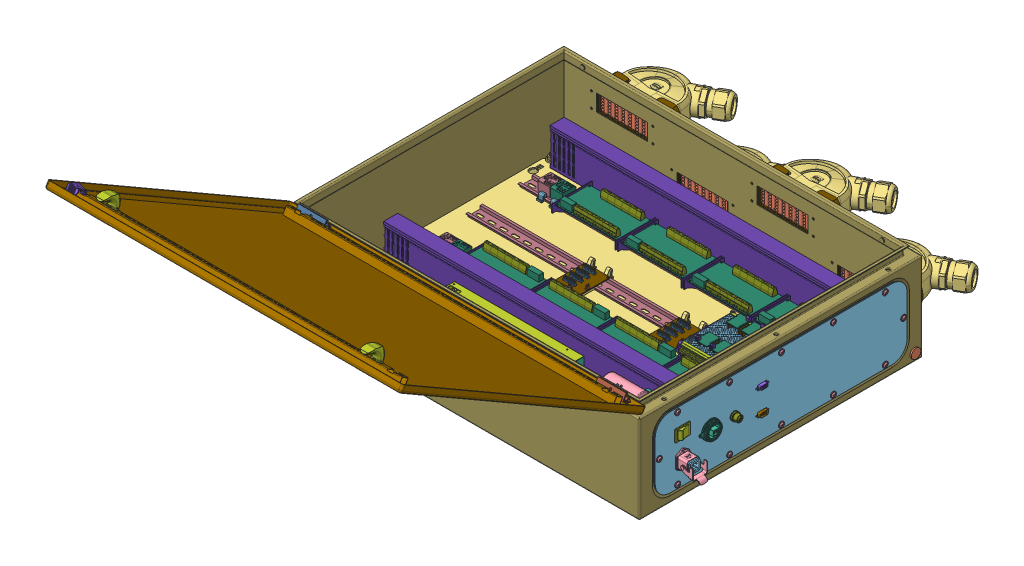
SolidWorks assembly _main_cabinet, configuration Default. Lengths in mm.
Overall size (807.06 524.8 1268.8).
399 component instances, 81 part files, 82 mates.
Components (placement in the parent):
- 1076_000_1_customized-1: 1076_000_1_customized [Default] x (0 0 -1) z (0 1 0) size (1110.24 763.7 524.8)
  - 1076_000_1__3-1: 1076_000_1__3 [Default] at (-280 360 -1.55) x (1 0 0) z (0 0 -1) size (15.5 15.5 6.5)
  - 1076_000_1__3-2: 1076_000_1__3 [Default] at (280 360 -1.55) x (1 0 0) z (0 0 -1) size (15.5 15.5 6.5)
  - 1076_000_1__3-3: 1076_000_1__3 [Default] at (-280 -360 -1.55) x (1 0 0) z (0 0 -1) size (15.5 15.5 6.5)
  - 1076_000_1__3-4: 1076_000_1__3 [Default] at (280 -360 -1.55) x (1 0 0) z (0 0 -1) size (15.5 15.5 6.5)
  - 1076_000_1__8-1: 1076_000_1__8 [Default] at (283.5 -380 16.5) size (20 6.85 20)
  - 1076_000_1__10-1: 1076_000_1__10 [Default] at (0 -355 20) size (550 735 2.5)
  - 1076_000_1__12-1: 1076_000_1__12 [Default] at (220 -379.25 160) x (1 0 0) z (0 0 -1) size (11.5 13.2 11.5)
  - 1076_000_1__12-2: 1076_000_1__12 [Default] at (110 -379.25 160) x (1 0 0) z (0 0 -1) size (11.5 13.2 11.5)
  - 1076_000_1__12-3: 1076_000_1__12 [Default] at (0 -379.25 160) x (1 0 0) z (0 0 -1) size (11.5 13.2 11.5)
  - 1076_000_1__12-4: 1076_000_1__12 [Default] at (-110 -379.25 160) x (1 0 0) z (0 0 -1) size (11.5 13.2 11.5)
  - 1076_000_1__12-5: 1076_000_1__12 [Default] at (-220 -379.25 160) x (1 0 0) z (0 0 -1) size (11.5 13.2 11.5)
  - 1076_000_1__12-6: 1076_000_1__12 [Default] at (220 -379.25 27) x (1 0 0) z (0 0 -1) size (11.5 13.2 11.5)
  - 1076_000_1__12-7: 1076_000_1__12 [Default] at (110 -379.25 27) x (1 0 0) z (0 0 -1) size (11.5 13.2 11.5)
  - 1076_000_1__12-8: 1076_000_1__12 [Default] at (0 -379.25 27) x (1 0 0) z (0 0 -1) size (11.5 13.2 11.5)
  - 1076_000_1__12-9: 1076_000_1__12 [Default] at (-110 -379.25 27) x (1 0 0) z (0 0 -1) size (11.5 13.2 11.5)
  - 1076_000_1__12-10: 1076_000_1__12 [Default] at (-220 -379.25 27) x (1 0 0) z (0 0 -1) size (11.5 13.2 11.5)
  - 1076_000_1__12-11: 1076_000_1__12 [Default] at (259 -379.25 93.5) x (1 0 0) z (0 0 -1) size (11.5 13.2 11.5)
  - 1076_000_1__12-12: 1076_000_1__12 [Default] at (-259 -379.25 93.5) x (1 0 0) z (0 0 -1) size (11.5 13.2 11.5)
  - 1076_000_1__25_customized-1: 1076_000_1__25_customized [Default] at (0 -380.5 93.5) size (534 1.5 149)
  - 1076_000_1__27-1: 1076_000_1__27 [Default] at (-278 -317.5 194.75) x (0 0 -1) z (0 1 0) size (10 7.19 10)
  - 1076_000_1__27-2: 1076_000_1__27 [Default] at (-278 317.5 194.75) x (0 0 -1) z (0 1 0) size (10 7.19 10)
  - Door^1076_000_1_customized-1: Door^1076_000_1_customized [Default] at (-443.434 0 518.2603) x (0.866025 0 -0.5) z (-0.5 0 -0.866025) size (595 755 52.01) (virtual)
    - 1076_000_1__30-1: 1076_000_1__30 [Default] at (-249.348 -280 210.722) x (1 0 0) z (0 -1 0) size (55.65 52.01 55.1)
    - 1076_000_1__30-2: 1076_000_1__30 [Default] at (-249.348 280 210.722) x (1 0 0) z (0 -1 0) size (55.65 52.01 55.1)
    - 1076_000_1__33-1: 1076_000_1__33 [Default] at (-262.098 -333 201.672) x (-1 0 0) z (0 0 -1) size (20.91 29.5 13.98)
    - 1076_000_1__35-1: 1076_000_1__35 [Default] at (-0.1395 1.3759 210.2049) size (595 755 17.5)
    - 1076_000_1__37-1: 1076_000_1__37 [Default] at (279.5 -317.5 194.75) x (0 0 1) z (1 0 0) size (16.07 66 15.75)
    - 1076_000_1__39-1: 1076_000_1__39 [Default] at (279.5 317.5 194.75) x (0 0 1) z (1 0 0) size (16.07 66 15.75)
  - 1076_000_1__41_customized-1: 1076_000_1__41_customized [Default] at (0 -380 105) size (600 760 205.1)
- DIN_rail_35x7.5_long-1: DIN_rail_35x7.5_long [Default] at (-340 20 -70) x (0 0 -1) z (1 0 0) size (35 7.5 680)
- DIN_rail_35x7.5_long-2: DIN_rail_35x7.5_long [Default] at (-340 20 -180) x (0 0 -1) z (1 0 0) size (35 7.5 680)
- DIN_rail_35x7.5_long-3: DIN_rail_35x7.5_long [Default] at (-340 20 40) x (0 0 -1) z (1 0 0) size (35 7.5 680)
- DIN_rail_35x7.5_psus-1: DIN_rail_35x7.5_psus [Default] at (247.5 20 125) size (35 7.5 150)
- Sanwo_16ch_mosfet_board-1: Sanwo_16ch_mosfet_board [Default] at (-242.3811 45.9 -143.9) size (136.5 36.9 85)
  - Sanwo_16ch_mosfet_board-1: Sanwo_16ch_mosfet_board [Default] at origin size (133.5 14.6 72.2)
  - screw_terminal_3x_large-1: screw_terminal_3x_large [Default] at (73.5 1.6 -64.7) size (15 18 10)
  - screw_terminal_3x_large-2: screw_terminal_3x_large [Default] at (103.5 1.6 -64.7) size (15 18 10)
  - screw_terminal_3x_large-3: screw_terminal_3x_large [Default] at (88.5 1.6 -64.7) size (15 18 10)
  - screw_terminal_3x_large-4: screw_terminal_3x_large [Default] at (58.5 1.6 -64.7) size (15 18 10)
  - screw_terminal_3x_large-5: screw_terminal_3x_large [Default] at (113.5 1.6 -64.7) size (15 18 10)
  - screw_terminal_3x_large-6: screw_terminal_3x_large [Default] at (43.5 1.6 -64.7) size (15 18 10)
  - screw_terminal_3x_large-7: screw_terminal_3x_large [Default] at (43.5 1.6 -7.5) x (-1 0 0) z (0 0 -1) size (15 18 10)
  - screw_terminal_3x_large-8: screw_terminal_3x_large [Default] at (103.5 1.6 -7.5) x (-1 0 0) z (0 0 -1) size (15 18 10)
  - screw_terminal_3x_large-9: screw_terminal_3x_large [Default] at (118.5 1.6 -7.5) x (-1 0 0) z (0 0 -1) size (15 18 10)
  - screw_terminal_3x_large-10: screw_terminal_3x_large [Default] at (73.5 1.6 -7.5) x (-1 0 0) z (0 0 -1) size (15 18 10)
  - screw_terminal_3x_large-11: screw_terminal_3x_large [Default] at (58.5 1.6 -7.5) x (-1 0 0) z (0 0 -1) size (15 18 10)
  - screw_terminal_3x_large-12: screw_terminal_3x_large [Default] at (88.5 1.6 -7.5) x (-1 0 0) z (0 0 -1) size (15 18 10)
  - Sanwo_16ch_mosfet_board_DIN_rail_support-1: Sanwo_16ch_mosfet_board_DIN_rail_support [Default] at (0 -18.4 -36.1) x (0 0 1) z (-1 0 0) size (85 26.2 1.5)
  - Sanwo_16ch_mosfet_board_DIN_rail_support-2: Sanwo_16ch_mosfet_board_DIN_rail_support [Default] at (135 -18.4 -36.1) x (0 0 1) z (-1 0 0) size (85 26.2 1.5)
- Sanwo_16ch_mosfet_board-2: Sanwo_16ch_mosfet_board [Default] at (-108.8811 45.9 3.9) x (-1 0 0) z (0 0 -1) size (136.5 36.9 85)
  - Sanwo_16ch_mosfet_board-1: Sanwo_16ch_mosfet_board [Default] at origin size (133.5 14.6 72.2)
  - screw_terminal_3x_large-1: screw_terminal_3x_large [Default] at (73.5 1.6 -64.7) size (15 18 10)
  - screw_terminal_3x_large-2: screw_terminal_3x_large [Default] at (103.5 1.6 -64.7) size (15 18 10)
  - screw_terminal_3x_large-3: screw_terminal_3x_large [Default] at (88.5 1.6 -64.7) size (15 18 10)
  - screw_terminal_3x_large-4: screw_terminal_3x_large [Default] at (58.5 1.6 -64.7) size (15 18 10)
  - screw_terminal_3x_large-5: screw_terminal_3x_large [Default] at (113.5 1.6 -64.7) size (15 18 10)
  - screw_terminal_3x_large-6: screw_terminal_3x_large [Default] at (43.5 1.6 -64.7) size (15 18 10)
  - screw_terminal_3x_large-7: screw_terminal_3x_large [Default] at (43.5 1.6 -7.5) x (-1 0 0) z (0 0 -1) size (15 18 10)
  - screw_terminal_3x_large-8: screw_terminal_3x_large [Default] at (103.5 1.6 -7.5) x (-1 0 0) z (0 0 -1) size (15 18 10)
  - screw_terminal_3x_large-9: screw_terminal_3x_large [Default] at (118.5 1.6 -7.5) x (-1 0 0) z (0 0 -1) size (15 18 10)
  - screw_terminal_3x_large-10: screw_terminal_3x_large [Default] at (73.5 1.6 -7.5) x (-1 0 0) z (0 0 -1) size (15 18 10)
  - screw_terminal_3x_large-11: screw_terminal_3x_large [Default] at (58.5 1.6 -7.5) x (-1 0 0) z (0 0 -1) size (15 18 10)
  - screw_terminal_3x_large-12: screw_terminal_3x_large [Default] at (88.5 1.6 -7.5) x (-1 0 0) z (0 0 -1) size (15 18 10)
  - Sanwo_16ch_mosfet_board_DIN_rail_support-1: Sanwo_16ch_mosfet_board_DIN_rail_support [Default] at (0 -18.4 -36.1) x (0 0 1) z (-1 0 0) size (85 26.2 1.5)
  - Sanwo_16ch_mosfet_board_DIN_rail_support-2: Sanwo_16ch_mosfet_board_DIN_rail_support [Default] at (135 -18.4 -36.1) x (0 0 1) z (-1 0 0) size (85 26.2 1.5)
- Sanwo_16ch_mosfet_board-3: Sanwo_16ch_mosfet_board [Default] at (31.1189 45.9 3.9) x (-1 0 0) z (0 0 -1) size (136.5 36.9 85)
  - Sanwo_16ch_mosfet_board-1: Sanwo_16ch_mosfet_board [Default] at origin size (133.5 14.6 72.2)
  - screw_terminal_3x_large-1: screw_terminal_3x_large [Default] at (73.5 1.6 -64.7) size (15 18 10)
  - screw_terminal_3x_large-2: screw_terminal_3x_large [Default] at (103.5 1.6 -64.7) size (15 18 10)
  - screw_terminal_3x_large-3: screw_terminal_3x_large [Default] at (88.5 1.6 -64.7) size (15 18 10)
  - screw_terminal_3x_large-4: screw_terminal_3x_large [Default] at (58.5 1.6 -64.7) size (15 18 10)
  - screw_terminal_3x_large-5: screw_terminal_3x_large [Default] at (113.5 1.6 -64.7) size (15 18 10)
  - screw_terminal_3x_large-6: screw_terminal_3x_large [Default] at (43.5 1.6 -64.7) size (15 18 10)
  - screw_terminal_3x_large-7: screw_terminal_3x_large [Default] at (43.5 1.6 -7.5) x (-1 0 0) z (0 0 -1) size (15 18 10)
  - screw_terminal_3x_large-8: screw_terminal_3x_large [Default] at (103.5 1.6 -7.5) x (-1 0 0) z (0 0 -1) size (15 18 10)
  - screw_terminal_3x_large-9: screw_terminal_3x_large [Default] at (118.5 1.6 -7.5) x (-1 0 0) z (0 0 -1) size (15 18 10)
  - screw_terminal_3x_large-10: screw_terminal_3x_large [Default] at (73.5 1.6 -7.5) x (-1 0 0) z (0 0 -1) size (15 18 10)
  - screw_terminal_3x_large-11: screw_terminal_3x_large [Default] at (58.5 1.6 -7.5) x (-1 0 0) z (0 0 -1) size (15 18 10)
  - screw_terminal_3x_large-12: screw_terminal_3x_large [Default] at (88.5 1.6 -7.5) x (-1 0 0) z (0 0 -1) size (15 18 10)
  - Sanwo_16ch_mosfet_board_DIN_rail_support-1: Sanwo_16ch_mosfet_board_DIN_rail_support [Default] at (0 -18.4 -36.1) x (0 0 1) z (-1 0 0) size (85 26.2 1.5)
  - Sanwo_16ch_mosfet_board_DIN_rail_support-2: Sanwo_16ch_mosfet_board_DIN_rail_support [Default] at (135 -18.4 -36.1) x (0 0 1) z (-1 0 0) size (85 26.2 1.5)
- Sanwo_16ch_mosfet_board-4: Sanwo_16ch_mosfet_board [Default] at (171.1189 45.9 3.9) x (-1 0 0) z (0 0 -1) size (136.5 36.9 85)
  - Sanwo_16ch_mosfet_board-1: Sanwo_16ch_mosfet_board [Default] at origin size (133.5 14.6 72.2)
  - screw_terminal_3x_large-1: screw_terminal_3x_large [Default] at (73.5 1.6 -64.7) size (15 18 10)
  - screw_terminal_3x_large-2: screw_terminal_3x_large [Default] at (103.5 1.6 -64.7) size (15 18 10)
  - screw_terminal_3x_large-3: screw_terminal_3x_large [Default] at (88.5 1.6 -64.7) size (15 18 10)
  - screw_terminal_3x_large-4: screw_terminal_3x_large [Default] at (58.5 1.6 -64.7) size (15 18 10)
  - screw_terminal_3x_large-5: screw_terminal_3x_large [Default] at (113.5 1.6 -64.7) size (15 18 10)
  - screw_terminal_3x_large-6: screw_terminal_3x_large [Default] at (43.5 1.6 -64.7) size (15 18 10)
  - screw_terminal_3x_large-7: screw_terminal_3x_large [Default] at (43.5 1.6 -7.5) x (-1 0 0) z (0 0 -1) size (15 18 10)
  - screw_terminal_3x_large-8: screw_terminal_3x_large [Default] at (103.5 1.6 -7.5) x (-1 0 0) z (0 0 -1) size (15 18 10)
  - screw_terminal_3x_large-9: screw_terminal_3x_large [Default] at (118.5 1.6 -7.5) x (-1 0 0) z (0 0 -1) size (15 18 10)
  - screw_terminal_3x_large-10: screw_terminal_3x_large [Default] at (73.5 1.6 -7.5) x (-1 0 0) z (0 0 -1) size (15 18 10)
  - screw_terminal_3x_large-11: screw_terminal_3x_large [Default] at (58.5 1.6 -7.5) x (-1 0 0) z (0 0 -1) size (15 18 10)
  - screw_terminal_3x_large-12: screw_terminal_3x_large [Default] at (88.5 1.6 -7.5) x (-1 0 0) z (0 0 -1) size (15 18 10)
  - Sanwo_16ch_mosfet_board_DIN_rail_support-1: Sanwo_16ch_mosfet_board_DIN_rail_support [Default] at (0 -18.4 -36.1) x (0 0 1) z (-1 0 0) size (85 26.2 1.5)
  - Sanwo_16ch_mosfet_board_DIN_rail_support-2: Sanwo_16ch_mosfet_board_DIN_rail_support [Default] at (135 -18.4 -36.1) x (0 0 1) z (-1 0 0) size (85 26.2 1.5)
- Sanwo_16ch_mosfet_board-5: Sanwo_16ch_mosfet_board [Default] at (311.1189 45.9 3.9) x (-1 0 0) z (0 0 -1) size (136.5 36.9 85)
  - Sanwo_16ch_mosfet_board-1: Sanwo_16ch_mosfet_board [Default] at origin size (133.5 14.6 72.2)
  - screw_terminal_3x_large-1: screw_terminal_3x_large [Default] at (73.5 1.6 -64.7) size (15 18 10)
  - screw_terminal_3x_large-2: screw_terminal_3x_large [Default] at (103.5 1.6 -64.7) size (15 18 10)
  - screw_terminal_3x_large-3: screw_terminal_3x_large [Default] at (88.5 1.6 -64.7) size (15 18 10)
  - screw_terminal_3x_large-4: screw_terminal_3x_large [Default] at (58.5 1.6 -64.7) size (15 18 10)
  - screw_terminal_3x_large-5: screw_terminal_3x_large [Default] at (113.5 1.6 -64.7) size (15 18 10)
  - screw_terminal_3x_large-6: screw_terminal_3x_large [Default] at (43.5 1.6 -64.7) size (15 18 10)
  - screw_terminal_3x_large-7: screw_terminal_3x_large [Default] at (43.5 1.6 -7.5) x (-1 0 0) z (0 0 -1) size (15 18 10)
  - screw_terminal_3x_large-8: screw_terminal_3x_large [Default] at (103.5 1.6 -7.5) x (-1 0 0) z (0 0 -1) size (15 18 10)
  - screw_terminal_3x_large-9: screw_terminal_3x_large [Default] at (118.5 1.6 -7.5) x (-1 0 0) z (0 0 -1) size (15 18 10)
  - screw_terminal_3x_large-10: screw_terminal_3x_large [Default] at (73.5 1.6 -7.5) x (-1 0 0) z (0 0 -1) size (15 18 10)
  - screw_terminal_3x_large-11: screw_terminal_3x_large [Default] at (58.5 1.6 -7.5) x (-1 0 0) z (0 0 -1) size (15 18 10)
  - screw_terminal_3x_large-12: screw_terminal_3x_large [Default] at (88.5 1.6 -7.5) x (-1 0 0) z (0 0 -1) size (15 18 10)
  - Sanwo_16ch_mosfet_board_DIN_rail_support-1: Sanwo_16ch_mosfet_board_DIN_rail_support [Default] at (0 -18.4 -36.1) x (0 0 1) z (-1 0 0) size (85 26.2 1.5)
  - Sanwo_16ch_mosfet_board_DIN_rail_support-2: Sanwo_16ch_mosfet_board_DIN_rail_support [Default] at (135 -18.4 -36.1) x (0 0 1) z (-1 0 0) size (85 26.2 1.5)
- Sanwo_16ch_mosfet_board-6: Sanwo_16ch_mosfet_board [Default] at (-102.3811 45.9 -143.9) size (136.5 36.9 85)
  - Sanwo_16ch_mosfet_board-1: Sanwo_16ch_mosfet_board [Default] at origin size (133.5 14.6 72.2)
  - screw_terminal_3x_large-1: screw_terminal_3x_large [Default] at (73.5 1.6 -64.7) size (15 18 10)
  - screw_terminal_3x_large-2: screw_terminal_3x_large [Default] at (103.5 1.6 -64.7) size (15 18 10)
  - screw_terminal_3x_large-3: screw_terminal_3x_large [Default] at (88.5 1.6 -64.7) size (15 18 10)
  - screw_terminal_3x_large-4: screw_terminal_3x_large [Default] at (58.5 1.6 -64.7) size (15 18 10)
  - screw_terminal_3x_large-5: screw_terminal_3x_large [Default] at (113.5 1.6 -64.7) size (15 18 10)
  - screw_terminal_3x_large-6: screw_terminal_3x_large [Default] at (43.5 1.6 -64.7) size (15 18 10)
  - screw_terminal_3x_large-7: screw_terminal_3x_large [Default] at (43.5 1.6 -7.5) x (-1 0 0) z (0 0 -1) size (15 18 10)
  - screw_terminal_3x_large-8: screw_terminal_3x_large [Default] at (103.5 1.6 -7.5) x (-1 0 0) z (0 0 -1) size (15 18 10)
  - screw_terminal_3x_large-9: screw_terminal_3x_large [Default] at (118.5 1.6 -7.5) x (-1 0 0) z (0 0 -1) size (15 18 10)
  - screw_terminal_3x_large-10: screw_terminal_3x_large [Default] at (73.5 1.6 -7.5) x (-1 0 0) z (0 0 -1) size (15 18 10)
  - screw_terminal_3x_large-11: screw_terminal_3x_large [Default] at (58.5 1.6 -7.5) x (-1 0 0) z (0 0 -1) size (15 18 10)
  - screw_terminal_3x_large-12: screw_terminal_3x_large [Default] at (88.5 1.6 -7.5) x (-1 0 0) z (0 0 -1) size (15 18 10)
  - Sanwo_16ch_mosfet_board_DIN_rail_support-1: Sanwo_16ch_mosfet_board_DIN_rail_support [Default] at (0 -18.4 -36.1) x (0 0 1) z (-1 0 0) size (85 26.2 1.5)
  - Sanwo_16ch_mosfet_board_DIN_rail_support-2: Sanwo_16ch_mosfet_board_DIN_rail_support [Default] at (135 -18.4 -36.1) x (0 0 1) z (-1 0 0) size (85 26.2 1.5)
- Sanwo_16ch_mosfet_board-7: Sanwo_16ch_mosfet_board [Default] at (37.6189 45.9 -143.9) size (136.5 36.9 85)
  - Sanwo_16ch_mosfet_board-1: Sanwo_16ch_mosfet_board [Default] at origin size (133.5 14.6 72.2)
  - screw_terminal_3x_large-1: screw_terminal_3x_large [Default] at (73.5 1.6 -64.7) size (15 18 10)
  - screw_terminal_3x_large-2: screw_terminal_3x_large [Default] at (103.5 1.6 -64.7) size (15 18 10)
  - screw_terminal_3x_large-3: screw_terminal_3x_large [Default] at (88.5 1.6 -64.7) size (15 18 10)
  - screw_terminal_3x_large-4: screw_terminal_3x_large [Default] at (58.5 1.6 -64.7) size (15 18 10)
  - screw_terminal_3x_large-5: screw_terminal_3x_large [Default] at (113.5 1.6 -64.7) size (15 18 10)
  - screw_terminal_3x_large-6: screw_terminal_3x_large [Default] at (43.5 1.6 -64.7) size (15 18 10)
  - screw_terminal_3x_large-7: screw_terminal_3x_large [Default] at (43.5 1.6 -7.5) x (-1 0 0) z (0 0 -1) size (15 18 10)
  - screw_terminal_3x_large-8: screw_terminal_3x_large [Default] at (103.5 1.6 -7.5) x (-1 0 0) z (0 0 -1) size (15 18 10)
  - screw_terminal_3x_large-9: screw_terminal_3x_large [Default] at (118.5 1.6 -7.5) x (-1 0 0) z (0 0 -1) size (15 18 10)
  - screw_terminal_3x_large-10: screw_terminal_3x_large [Default] at (73.5 1.6 -7.5) x (-1 0 0) z (0 0 -1) size (15 18 10)
  - screw_terminal_3x_large-11: screw_terminal_3x_large [Default] at (58.5 1.6 -7.5) x (-1 0 0) z (0 0 -1) size (15 18 10)
  - screw_terminal_3x_large-12: screw_terminal_3x_large [Default] at (88.5 1.6 -7.5) x (-1 0 0) z (0 0 -1) size (15 18 10)
  - Sanwo_16ch_mosfet_board_DIN_rail_support-1: Sanwo_16ch_mosfet_board_DIN_rail_support [Default] at (0 -18.4 -36.1) x (0 0 1) z (-1 0 0) size (85 26.2 1.5)
  - Sanwo_16ch_mosfet_board_DIN_rail_support-2: Sanwo_16ch_mosfet_board_DIN_rail_support [Default] at (135 -18.4 -36.1) x (0 0 1) z (-1 0 0) size (85 26.2 1.5)
- Sanwo_16ch_mosfet_board-8: Sanwo_16ch_mosfet_board [Default] at (177.6189 45.9 -143.9) size (136.5 36.9 85)
  - Sanwo_16ch_mosfet_board-1: Sanwo_16ch_mosfet_board [Default] at origin size (133.5 14.6 72.2)
  - screw_terminal_3x_large-1: screw_terminal_3x_large [Default] at (73.5 1.6 -64.7) size (15 18 10)
  - screw_terminal_3x_large-2: screw_terminal_3x_large [Default] at (103.5 1.6 -64.7) size (15 18 10)
  - screw_terminal_3x_large-3: screw_terminal_3x_large [Default] at (88.5 1.6 -64.7) size (15 18 10)
  - screw_terminal_3x_large-4: screw_terminal_3x_large [Default] at (58.5 1.6 -64.7) size (15 18 10)
  - screw_terminal_3x_large-5: screw_terminal_3x_large [Default] at (113.5 1.6 -64.7) size (15 18 10)
  - screw_terminal_3x_large-6: screw_terminal_3x_large [Default] at (43.5 1.6 -64.7) size (15 18 10)
  - screw_terminal_3x_large-7: screw_terminal_3x_large [Default] at (43.5 1.6 -7.5) x (-1 0 0) z (0 0 -1) size (15 18 10)
  - screw_terminal_3x_large-8: screw_terminal_3x_large [Default] at (103.5 1.6 -7.5) x (-1 0 0) z (0 0 -1) size (15 18 10)
  - screw_terminal_3x_large-9: screw_terminal_3x_large [Default] at (118.5 1.6 -7.5) x (-1 0 0) z (0 0 -1) size (15 18 10)
  - screw_terminal_3x_large-10: screw_terminal_3x_large [Default] at (73.5 1.6 -7.5) x (-1 0 0) z (0 0 -1) size (15 18 10)
  - screw_terminal_3x_large-11: screw_terminal_3x_large [Default] at (58.5 1.6 -7.5) x (-1 0 0) z (0 0 -1) size (15 18 10)
  - screw_terminal_3x_large-12: screw_terminal_3x_large [Default] at (88.5 1.6 -7.5) x (-1 0 0) z (0 0 -1) size (15 18 10)
  - Sanwo_16ch_mosfet_board_DIN_rail_support-1: Sanwo_16ch_mosfet_board_DIN_rail_support [Default] at (0 -18.4 -36.1) x (0 0 1) z (-1 0 0) size (85 26.2 1.5)
  - Sanwo_16ch_mosfet_board_DIN_rail_support-2: Sanwo_16ch_mosfet_board_DIN_rail_support [Default] at (135 -18.4 -36.1) x (0 0 1) z (-1 0 0) size (85 26.2 1.5)
- Harting Mod.24-HSE-M40-1: Harting Mod.24-HSE-M40 [Default] at (-255 123.75 -322) x (1 0 0) z (0 1 0) size (185.57 158.35 76.54)
  - 19410240301_100198179MOD000C-HOUSING-1: 19410240301_100198179MOD000C-HOUSING [Default] at origin size (154.05 52.02 60.84)
  - 09140052601_100548017MOD000C.stp-1: 09140052601_100548017MOD000C.stp [Default] at (-43.15 34.9 0) x (-1 0 0) z (0 -1 0) size (14.7 34.2 34.4)
  - 09140052701_100548140MOD000C-1: 09140052701_100548140MOD000C [Default] at (-43.15 -15.2 0) x (1 0 0) z (0 1 0) size (14.7 34.2 36.4)
  - 19411240523_100556387MOD000C-HOUSING-1: 19411240523_100556387MOD000C-HOUSING [Default] at (1.9 -19.75 0) x (1 0 0) z (0 1 0) size (167.15 76.54 124.97)
  - 09140052701_100548140MOD000C-2: 09140052701_100548140MOD000C [Default] at (-28.65 -15.2 0) x (1 0 0) z (0 1 0) size (14.7 34.2 36.4)
  - 09140052701_100548140MOD000C-3: 09140052701_100548140MOD000C [Default] at (-14.15 -15.2 0) x (1 0 0) z (0 1 0) size (14.7 34.2 36.4)
  - 09140052701_100548140MOD000C-4: 09140052701_100548140MOD000C [Default] at (0.35 -15.2 0) x (1 0 0) z (0 1 0) size (14.7 34.2 36.4)
  - 09140052701_100548140MOD000C-5: 09140052701_100548140MOD000C [Default] at (14.85 -15.2 0) x (1 0 0) z (0 1 0) size (14.7 34.2 36.4)
  - 09140052701_100548140MOD000C-6: 09140052701_100548140MOD000C [Default] at (29.35 -15.2 0) x (1 0 0) z (0 1 0) size (14.7 34.2 36.4)
  - 09140052701_100548140MOD000C-7: 09140052701_100548140MOD000C [Default] at (43.85 -15.2 0) x (1 0 0) z (0 1 0) size (14.7 34.2 36.4)
  - 09140052601_100548017MOD000C.stp-2: 09140052601_100548017MOD000C.stp [Default] at (-28.65 34.9 0) x (-1 0 0) z (0 -1 0) size (14.7 34.2 34.4)
  - 09140052601_100548017MOD000C.stp-3: 09140052601_100548017MOD000C.stp [Default] at (-14.15 34.9 0) x (-1 0 0) z (0 -1 0) size (14.7 34.2 34.4)
  - 09140052601_100548017MOD000C.stp-4: 09140052601_100548017MOD000C.stp [Default] at (0.35 34.9 0) x (-1 0 0) z (0 -1 0) size (14.7 34.2 34.4)
  - 09140052601_100548017MOD000C.stp-5: 09140052601_100548017MOD000C.stp [Default] at (14.85 34.9 0) x (-1 0 0) z (0 -1 0) size (14.7 34.2 34.4)
  - 09140052601_100548017MOD000C.stp-6: 09140052601_100548017MOD000C.stp [Default] at (29.35 34.9 0) x (-1 0 0) z (0 -1 0) size (14.7 34.2 34.4)
  - 09140052601_100548017MOD000C.stp-7: 09140052601_100548017MOD000C.stp [Default] at (43.85 34.9 0) x (-1 0 0) z (0 -1 0) size (14.7 34.2 34.4)
- Harting Mod.24-HSE-M40-14: Harting Mod.24-HSE-M40 [Default] at (-85 63.75 -322) x (1 0 0) z (0 1 0) size (185.57 158.35 76.54)
  - 19410240301_100198179MOD000C-HOUSING-1: 19410240301_100198179MOD000C-HOUSING [Default] at origin size (154.05 52.02 60.84)
  - 09140052601_100548017MOD000C.stp-1: 09140052601_100548017MOD000C.stp [Default] at (-43.15 34.9 0) x (-1 0 0) z (0 -1 0) size (14.7 34.2 34.4)
  - 09140052701_100548140MOD000C-1: 09140052701_100548140MOD000C [Default] at (-43.15 -15.2 0) x (1 0 0) z (0 1 0) size (14.7 34.2 36.4)
  - 19411240523_100556387MOD000C-HOUSING-1: 19411240523_100556387MOD000C-HOUSING [Default] at (1.9 -19.75 0) x (1 0 0) z (0 1 0) size (167.15 76.54 124.97)
  - 09140052701_100548140MOD000C-2: 09140052701_100548140MOD000C [Default] at (-28.65 -15.2 0) x (1 0 0) z (0 1 0) size (14.7 34.2 36.4)
  - 09140052701_100548140MOD000C-3: 09140052701_100548140MOD000C [Default] at (-14.15 -15.2 0) x (1 0 0) z (0 1 0) size (14.7 34.2 36.4)
  - 09140052701_100548140MOD000C-4: 09140052701_100548140MOD000C [Default] at (0.35 -15.2 0) x (1 0 0) z (0 1 0) size (14.7 34.2 36.4)
  - 09140052701_100548140MOD000C-5: 09140052701_100548140MOD000C [Default] at (14.85 -15.2 0) x (1 0 0) z (0 1 0) size (14.7 34.2 36.4)
  - 09140052701_100548140MOD000C-6: 09140052701_100548140MOD000C [Default] at (29.35 -15.2 0) x (1 0 0) z (0 1 0) size (14.7 34.2 36.4)
  - 09140052701_100548140MOD000C-7: 09140052701_100548140MOD000C [Default] at (43.85 -15.2 0) x (1 0 0) z (0 1 0) size (14.7 34.2 36.4)
  - 09140052601_100548017MOD000C.stp-2: 09140052601_100548017MOD000C.stp [Default] at (-28.65 34.9 0) x (-1 0 0) z (0 -1 0) size (14.7 34.2 34.4)
  - 09140052601_100548017MOD000C.stp-3: 09140052601_100548017MOD000C.stp [Default] at (-14.15 34.9 0) x (-1 0 0) z (0 -1 0) size (14.7 34.2 34.4)
  - 09140052601_100548017MOD000C.stp-4: 09140052601_100548017MOD000C.stp [Default] at (0.35 34.9 0) x (-1 0 0) z (0 -1 0) size (14.7 34.2 34.4)
  - 09140052601_100548017MOD000C.stp-5: 09140052601_100548017MOD000C.stp [Default] at (14.85 34.9 0) x (-1 0 0) z (0 -1 0) size (14.7 34.2 34.4)
  - 09140052601_100548017MOD000C.stp-6: 09140052601_100548017MOD000C.stp [Default] at (29.35 34.9 0) x (-1 0 0) z (0 -1 0) size (14.7 34.2 34.4)
  - 09140052601_100548017MOD000C.stp-7: 09140052601_100548017MOD000C.stp [Default] at (43.85 34.9 0) x (-1 0 0) z (0 -1 0) size (14.7 34.2 34.4)
- Harting Mod.24-HSE-M40-15: Harting Mod.24-HSE-M40 [Default] at (85 123.75 -322) x (1 0 0) z (0 1 0) size (185.57 158.35 76.54)
  - 19410240301_100198179MOD000C-HOUSING-1: 19410240301_100198179MOD000C-HOUSING [Default] at origin size (154.05 52.02 60.84)
  - 09140052601_100548017MOD000C.stp-1: 09140052601_100548017MOD000C.stp [Default] at (-43.15 34.9 0) x (-1 0 0) z (0 -1 0) size (14.7 34.2 34.4)
  - 09140052701_100548140MOD000C-1: 09140052701_100548140MOD000C [Default] at (-43.15 -15.2 0) x (1 0 0) z (0 1 0) size (14.7 34.2 36.4)
  - 19411240523_100556387MOD000C-HOUSING-1: 19411240523_100556387MOD000C-HOUSING [Default] at (1.9 -19.75 0) x (1 0 0) z (0 1 0) size (167.15 76.54 124.97)
  - 09140052701_100548140MOD000C-2: 09140052701_100548140MOD000C [Default] at (-28.65 -15.2 0) x (1 0 0) z (0 1 0) size (14.7 34.2 36.4)
  - 09140052701_100548140MOD000C-3: 09140052701_100548140MOD000C [Default] at (-14.15 -15.2 0) x (1 0 0) z (0 1 0) size (14.7 34.2 36.4)
  - 09140052701_100548140MOD000C-4: 09140052701_100548140MOD000C [Default] at (0.35 -15.2 0) x (1 0 0) z (0 1 0) size (14.7 34.2 36.4)
  - 09140052701_100548140MOD000C-5: 09140052701_100548140MOD000C [Default] at (14.85 -15.2 0) x (1 0 0) z (0 1 0) size (14.7 34.2 36.4)
  - 09140052701_100548140MOD000C-6: 09140052701_100548140MOD000C [Default] at (29.35 -15.2 0) x (1 0 0) z (0 1 0) size (14.7 34.2 36.4)
  - 09140052701_100548140MOD000C-7: 09140052701_100548140MOD000C [Default] at (43.85 -15.2 0) x (1 0 0) z (0 1 0) size (14.7 34.2 36.4)
  - 09140052601_100548017MOD000C.stp-2: 09140052601_100548017MOD000C.stp [Default] at (-28.65 34.9 0) x (-1 0 0) z (0 -1 0) size (14.7 34.2 34.4)
  - 09140052601_100548017MOD000C.stp-3: 09140052601_100548017MOD000C.stp [Default] at (-14.15 34.9 0) x (-1 0 0) z (0 -1 0) size (14.7 34.2 34.4)
  - 09140052601_100548017MOD000C.stp-4: 09140052601_100548017MOD000C.stp [Default] at (0.35 34.9 0) x (-1 0 0) z (0 -1 0) size (14.7 34.2 34.4)
  - 09140052601_100548017MOD000C.stp-5: 09140052601_100548017MOD000C.stp [Default] at (14.85 34.9 0) x (-1 0 0) z (0 -1 0) size (14.7 34.2 34.4)
  - 09140052601_100548017MOD000C.stp-6: 09140052601_100548017MOD000C.stp [Default] at (29.35 34.9 0) x (-1 0 0) z (0 -1 0) size (14.7 34.2 34.4)
  - 09140052601_100548017MOD000C.stp-7: 09140052601_100548017MOD000C.stp [Default] at (43.85 34.9 0) x (-1 0 0) z (0 -1 0) size (14.7 34.2 34.4)
- Harting Mod.24-HSE-M40-16: Harting Mod.24-HSE-M40 [Default] at (255 63.75 -322) x (1 0 0) z (0 1 0) size (185.57 158.35 76.54)
  - 19410240301_100198179MOD000C-HOUSING-1: 19410240301_100198179MOD000C-HOUSING [Default] at origin size (154.05 52.02 60.84)
  - 09140052601_100548017MOD000C.stp-1: 09140052601_100548017MOD000C.stp [Default] at (-43.15 34.9 0) x (-1 0 0) z (0 -1 0) size (14.7 34.2 34.4)
  - 09140052701_100548140MOD000C-1: 09140052701_100548140MOD000C [Default] at (-43.15 -15.2 0) x (1 0 0) z (0 1 0) size (14.7 34.2 36.4)
  - 19411240523_100556387MOD000C-HOUSING-1: 19411240523_100556387MOD000C-HOUSING [Default] at (1.9 -19.75 0) x (1 0 0) z (0 1 0) size (167.15 76.54 124.97)
  - 09140052701_100548140MOD000C-2: 09140052701_100548140MOD000C [Default] at (-28.65 -15.2 0) x (1 0 0) z (0 1 0) size (14.7 34.2 36.4)
  - 09140052701_100548140MOD000C-3: 09140052701_100548140MOD000C [Default] at (-14.15 -15.2 0) x (1 0 0) z (0 1 0) size (14.7 34.2 36.4)
  - 09140052701_100548140MOD000C-4: 09140052701_100548140MOD000C [Default] at (0.35 -15.2 0) x (1 0 0) z (0 1 0) size (14.7 34.2 36.4)
  - 09140052701_100548140MOD000C-5: 09140052701_100548140MOD000C [Default] at (14.85 -15.2 0) x (1 0 0) z (0 1 0) size (14.7 34.2 36.4)
  - 09140052701_100548140MOD000C-6: 09140052701_100548140MOD000C [Default] at (29.35 -15.2 0) x (1 0 0) z (0 1 0) size (14.7 34.2 36.4)
  - 09140052701_100548140MOD000C-7: 09140052701_100548140MOD000C [Default] at (43.85 -15.2 0) x (1 0 0) z (0 1 0) size (14.7 34.2 36.4)
  - 09140052601_100548017MOD000C.stp-2: 09140052601_100548017MOD000C.stp [Default] at (-28.65 34.9 0) x (-1 0 0) z (0 -1 0) size (14.7 34.2 34.4)
  - 09140052601_100548017MOD000C.stp-3: 09140052601_100548017MOD000C.stp [Default] at (-14.15 34.9 0) x (-1 0 0) z (0 -1 0) size (14.7 34.2 34.4)
  - 09140052601_100548017MOD000C.stp-4: 09140052601_100548017MOD000C.stp [Default] at (0.35 34.9 0) x (-1 0 0) z (0 -1 0) size (14.7 34.2 34.4)
  - 09140052601_100548017MOD000C.stp-5: 09140052601_100548017MOD000C.stp [Default] at (14.85 34.9 0) x (-1 0 0) z (0 -1 0) size (14.7 34.2 34.4)
  - 09140052601_100548017MOD000C.stp-6: 09140052601_100548017MOD000C.stp [Default] at (29.35 34.9 0) x (-1 0 0) z (0 -1 0) size (14.7 34.2 34.4)
  - 09140052601_100548017MOD000C.stp-7: 09140052601_100548017MOD000C.stp [Default] at (43.85 34.9 0) x (-1 0 0) z (0 -1 0) size (14.7 34.2 34.4)
- DNR30_60-1: DNR30_60 [Default] at (253.3345 -2.4064 200.95) x (-1 0 0) z (0 0 -1) size (88.92 121.82 41.32)
- CUI_PSK-10D-3-DIN-1: CUI_PSK-10D-3-DIN [Default] at (249 28.5 163.7) x (-1 0 0) z (0 0 -1) size (76.02 34.4 31.52)
- txln750_3D_drawing^_main_cabinet-1: txln750_3D_drawing^_main_cabinet [Default] at (-34.7816 83.2954 180) x (0 0 -1) z (1 0 0) size (125 63 298.85) (virtual)
  - CASE^txln750_3D_drawing__main_cabinet-1: CASE^txln750_3D_drawing__main_cabinet [Default] at (-22.1168 -63.2954 0) size (124.2 62.2 274.2) (virtual)
  - COVER^txln750_3D_drawing__main_cabinet-1: COVER^txln750_3D_drawing__main_cabinet [Default] at (-21.6168 -1.0954 -0.5) size (124.8 62.8 274.8) (virtual)
  - FAN GUARD^txln750_3D_drawing__main_cabinet-1: FAN GUARD^txln750_3D_drawing__main_cabinet [Default] at (-42.2168 -31.8954 137.9) x (0 -1 0) z (-1 0 0) size (57.87 8.11 57.87) (virtual)
  - FAN60x25^txln750_3D_drawing__main_cabinet-1: FAN60x25^txln750_3D_drawing__main_cabinet [Default] at (-42.2168 -31.8954 123.6) size (60 60 25) (virtual)
  - PCB^txln750_3D_drawing__main_cabinet-1: PCB^txln750_3D_drawing__main_cabinet [Default] at (37.6923 -59.2954 134.8634) x (0 0 -1) z (0 1 0) size (270.48 120 1.6) (virtual)
  - TML BLK1^txln750_3D_drawing__main_cabinet-1: TML BLK1^txln750_3D_drawing__main_cabinet [Default] at (-0.9417 -50.1454 130.1001) size (34.5 18.1 23.6) (virtual)
  - TML BLK2^txln750_3D_drawing__main_cabinet-1: TML BLK2^txln750_3D_drawing__main_cabinet [Default] at (3.9832 -47.1954 -130.2504) x (-1 0 0) z (0 0 -1) size (68.6 22.4 32.6) (virtual)
  - HOUSING^txln750_3D_drawing__main_cabinet-1: HOUSING^txln750_3D_drawing__main_cabinet [Default] at (26.2332 -19.7954 -132.5) x (0 -1 0) z (0 0 -1) size (10 5.1 8.64) (virtual)
- custom_perfboard-1: custom_perfboard [Default] at (151.5551 53.8 -20.003) size (162 55.7 125.4)
  - perfboard-1: perfboard [Default] at origin size (160 1.6 100)
  - 4-20mA_R_click_in_headers-1: 4-20mA_R_click_in_headers [Default] at (22.87 12.6 -69.05) size (25.4 24.5 30.48)
    - 4-20mA_R_click-1: 4-20mA_R_click [Default] at origin size (25.4 1.7 30.48)
    - header_m8-1: header_m8 [Default] at (1.25 -2.5 -22.86) x (0 0 1) z (-1 0 0) size (20.32 11.5 2.5)
    - header_m8-2: header_m8 [Default] at (24.15 -2.5 -2.54) x (0 0 -1) z (1 0 0) size (20.32 11.5 2.5)
    - screw_terminal_2x_2.54pitch-1: screw_terminal_2x_2.54pitch [Default] at (24.765 1.7 -23.545) x (0 0 -1) z (1 0 0) size (6.3 12.6 5.6)
    - header_f8-1: header_f8 [Default] at (24.15 -11 -2.415) x (0 0 -1) z (1 0 0) size (20.57 11.5 2.5)
    - header_f8-2: header_f8 [Default] at (1.25 -11 -22.985) x (0 0 1) z (-1 0 0) size (20.57 11.5 2.5)
  - 4-20mA_R_click_in_headers-5: 4-20mA_R_click_in_headers [Default] at (48.27 12.6 -33.49) x (-1 0 0) z (0 0 -1) size (25.4 24.5 30.48)
    - 4-20mA_R_click-1: 4-20mA_R_click [Default] at origin size (25.4 1.7 30.48)
    - header_m8-1: header_m8 [Default] at (1.25 -2.5 -22.86) x (0 0 1) z (-1 0 0) size (20.32 11.5 2.5)
    - header_m8-2: header_m8 [Default] at (24.15 -2.5 -2.54) x (0 0 -1) z (1 0 0) size (20.32 11.5 2.5)
    - screw_terminal_2x_2.54pitch-1: screw_terminal_2x_2.54pitch [Default] at (24.765 1.7 -23.545) x (0 0 -1) z (1 0 0) size (6.3 12.6 5.6)
    - header_f8-1: header_f8 [Default] at (24.15 -11 -2.415) x (0 0 -1) z (1 0 0) size (20.57 11.5 2.5)
    - header_f8-2: header_f8 [Default] at (1.25 -11 -22.985) x (0 0 1) z (-1 0 0) size (20.57 11.5 2.5)
  - 4-20mA_R_click_in_headers-2: 4-20mA_R_click_in_headers [Default] at (53.35 12.6 -69.05) size (25.4 24.5 30.48)
    - 4-20mA_R_click-1: 4-20mA_R_click [Default] at origin size (25.4 1.7 30.48)
    - header_m8-1: header_m8 [Default] at (1.25 -2.5 -22.86) x (0 0 1) z (-1 0 0) size (20.32 11.5 2.5)
    - header_m8-2: header_m8 [Default] at (24.15 -2.5 -2.54) x (0 0 -1) z (1 0 0) size (20.32 11.5 2.5)
    - screw_terminal_2x_2.54pitch-1: screw_terminal_2x_2.54pitch [Default] at (24.765 1.7 -23.545) x (0 0 -1) z (1 0 0) size (6.3 12.6 5.6)
    - header_f8-1: header_f8 [Default] at (24.15 -11 -2.415) x (0 0 -1) z (1 0 0) size (20.57 11.5 2.5)
    - header_f8-2: header_f8 [Default] at (1.25 -11 -22.985) x (0 0 1) z (-1 0 0) size (20.57 11.5 2.5)
  - 3857 Adafruit Feather M4 Express headers 2-1: 3857 Adafruit Feather M4 Express headers 2 [Default] at (160.01 12.6 -94.45) x (-1 0 0) z (0 1 0) size (50.85 22.86 20.37)
    - 3857 Adafruit Feather M4 Express-1: 3857 Adafruit Feather M4 Express [Default] at origin size (50.85 22.86 6.37)
      - 3857 Adafruit Feather M4 Express(2)^3857 Adafruit Feather M4 Express-1: 3857 Adafruit Feather M4 Express(2)^3857 Adafruit Feather M4 Express [Default] at origin size (50.85 22.86 6.37) (virtual)
        - PCB Component^3857 Adafruit Feather M4 Express(2)_3857 Adafruit Feather M4 Express-1: PCB Component^3857 Adafruit Feather M4 Express(2)_3857 Adafruit Feather M4 Express [Default] at origin size (50.85 22.86 6.37) (virtual)
          - Board^PCB Component_3857 Adafruit Feather M4 Express(2)_3857 Adafruit Feather M4 Express-1: Board^PCB Component_3857 Adafruit Feather M4 Express(2)_3857 Adafruit Feather M4 Express [Default] at origin size (50.8 22.86 1.57) (virtual)
          - 10uF^PCB Component_3857 Adafruit Feather M4 Express(2)_3857 Adafruit Feather M4 Express-1: 10uF^PCB Component_3857 Adafruit Feather M4 Express(2)_3857 Adafruit Feather M4 Express [Default] at (12.042 9.838 1.57) x (0 -1 0) z (0 0 1) size (2 1.25 1) (virtual)
          - 10uF^PCB Component_3857 Adafruit Feather M4 Express(2)_3857 Adafruit Feather M4 Express-2: 10uF^PCB Component_3857 Adafruit Feather M4 Express(2)_3857 Adafruit Feather M4 Express [Default] at (14.728 13.858 1.57) size (2 1.25 1) (virtual)
          - 10uF^PCB Component_3857 Adafruit Feather M4 Express(2)_3857 Adafruit Feather M4 Express-3: 10uF^PCB Component_3857 Adafruit Feather M4 Express(2)_3857 Adafruit Feather M4 Express [Default] at (15.748 17.272 1.57) x (0 -1 0) z (0 0 1) size (2 1.25 1) (virtual)
          - 10uF^PCB Component_3857 Adafruit Feather M4 Express(2)_3857 Adafruit Feather M4 Express-4: 10uF^PCB Component_3857 Adafruit Feather M4 Express(2)_3857 Adafruit Feather M4 Express [Default] at (35.065 18.669 1.57) size (2 1.25 1) (virtual)
          - 10uF^PCB Component_3857 Adafruit Feather M4 Express(2)_3857 Adafruit Feather M4 Express-5: 10uF^PCB Component_3857 Adafruit Feather M4 Express(2)_3857 Adafruit Feather M4 Express [Default] at (18.796 11.303 1.57) x (0 -1 0) z (0 0 1) size (2 1.25 1) (virtual)
          - 1uF^PCB Component_3857 Adafruit Feather M4 Express(2)_3857 Adafruit Feather M4 Express-1: 1uF^PCB Component_3857 Adafruit Feather M4 Express(2)_3857 Adafruit Feather M4 Express [Default] at (24.909 17.78 1.57) x (0 1 0) z (0 0 1) size (1.6 0.9 0.8) (virtual)
          - 1uF^PCB Component_3857 Adafruit Feather M4 Express(2)_3857 Adafruit Feather M4 Express-2: 1uF^PCB Component_3857 Adafruit Feather M4 Express(2)_3857 Adafruit Feather M4 Express [Default] at (11.989 4.218 1.57) size (1.6 0.9 0.8) (virtual)
          - 1uF^PCB Component_3857 Adafruit Feather M4 Express(2)_3857 Adafruit Feather M4 Express-3: 1uF^PCB Component_3857 Adafruit Feather M4 Express(2)_3857 Adafruit Feather M4 Express [Default] at (5.715 20.955 1.57) x (0 -1 0) z (0 0 1) size (1.6 0.9 0.8) (virtual)
          - 1uF^PCB Component_3857 Adafruit Feather M4 Express(2)_3857 Adafruit Feather M4 Express-4: 1uF^PCB Component_3857 Adafruit Feather M4 Express(2)_3857 Adafruit Feather M4 Express [Default] at (5.829 4.254 1.57) size (1.6 0.9 0.8) (virtual)
          - 1uF^PCB Component_3857 Adafruit Feather M4 Express(2)_3857 Adafruit Feather M4 Express-5: 1uF^PCB Component_3857 Adafruit Feather M4 Express(2)_3857 Adafruit Feather M4 Express [Default] at (18.415 17.97 1.57) size (1.6 0.9 0.8) (virtual)
          - 1uF^PCB Component_3857 Adafruit Feather M4 Express(2)_3857 Adafruit Feather M4 Express-6: 1uF^PCB Component_3857 Adafruit Feather M4 Express(2)_3857 Adafruit Feather M4 Express [Default] at (19.202 5.067 1.57) x (0 1 0) z (0 0 1) size (1.6 0.9 0.8) (virtual)
          - 1uF^PCB Component_3857 Adafruit Feather M4 Express(2)_3857 Adafruit Feather M4 Express-7: 1uF^PCB Component_3857 Adafruit Feather M4 Express(2)_3857 Adafruit Feather M4 Express [Default] at (21.526 6.35 1.57) x (-1 0 0) z (0 0 1) size (1.6 0.9 0.8) (virtual)
          - 1uF^PCB Component_3857 Adafruit Feather M4 Express(2)_3857 Adafruit Feather M4 Express-8: 1uF^PCB Component_3857 Adafruit Feather M4 Express(2)_3857 Adafruit Feather M4 Express [Default] at (36.119 4.648 1.57) x (-1 0 0) z (0 0 1) size (1.6 0.9 0.8) (virtual)
          - 1uF^PCB Component_3857 Adafruit Feather M4 Express(2)_3857 Adafruit Feather M4 Express-9: 1uF^PCB Component_3857 Adafruit Feather M4 Express(2)_3857 Adafruit Feather M4 Express [Default] at (19.126 8.065 1.57) x (0 1 0) z (0 0 1) size (1.6 0.9 0.8) (virtual)
          - 1uF^PCB Component_3857 Adafruit Feather M4 Express(2)_3857 Adafruit Feather M4 Express-10: 1uF^PCB Component_3857 Adafruit Feather M4 Express(2)_3857 Adafruit Feather M4 Express [Default] at (29.662 5.263 1.57) x (-1 0 0) z (0 0 1) size (1.6 0.9 0.8) (virtual)
          - 1uF^PCB Component_3857 Adafruit Feather M4 Express(2)_3857 Adafruit Feather M4 Express-11: 1uF^PCB Component_3857 Adafruit Feather M4 Express(2)_3857 Adafruit Feather M4 Express [Default] at (8.89 4.254 1.57) x (-1 0 0) z (0 0 1) size (1.6 0.9 0.8) (virtual)
          - 1uF^PCB Component_3857 Adafruit Feather M4 Express(2)_3857 Adafruit Feather M4 Express-12: 1uF^PCB Component_3857 Adafruit Feather M4 Express(2)_3857 Adafruit Feather M4 Express [Default] at (17.145 10.922 1.57) x (0 1 0) z (0 0 1) size (1.6 0.9 0.8) (virtual)
          - 1uF^PCB Component_3857 Adafruit Feather M4 Express(2)_3857 Adafruit Feather M4 Express-13: 1uF^PCB Component_3857 Adafruit Feather M4 Express(2)_3857 Adafruit Feather M4 Express [Default] at (13.856 6.502 1.57) x (0 -1 0) z (0 0 1) size (1.6 0.9 0.8) (virtual)
          - 1uF^PCB Component_3857 Adafruit Feather M4 Express(2)_3857 Adafruit Feather M4 Express-14: 1uF^PCB Component_3857 Adafruit Feather M4 Express(2)_3857 Adafruit Feather M4 Express [Default] at (21.4 8.065 1.57) size (1.6 0.9 0.8) (virtual)
          - 1uF^PCB Component_3857 Adafruit Feather M4 Express(2)_3857 Adafruit Feather M4 Express-15: 1uF^PCB Component_3857 Adafruit Feather M4 Express(2)_3857 Adafruit Feather M4 Express [Default] at (22.225 14.414 1.57) x (-1 0 0) z (0 0 1) size (1.6 0.9 0.8) (virtual)
          - ORANGE^PCB Component_3857 Adafruit Feather M4 Express(2)_3857 Adafruit Feather M4 Express-1: ORANGE^PCB Component_3857 Adafruit Feather M4 Express(2)_3857 Adafruit Feather M4 Express [Default] at (2.645 17.359 1.57) x (0 1 0) z (0 0 1) size (1.25 2.02 1.1) (virtual)
          - ORANGE^PCB Component_3857 Adafruit Feather M4 Express(2)_3857 Adafruit Feather M4 Express-2: ORANGE^PCB Component_3857 Adafruit Feather M4 Express(2)_3857 Adafruit Feather M4 Express [Default] at (2.413 5.588 1.57) x (0 -1 0) z (0 0 1) size (1.25 2.02 1.1) (virtual)
          - KMR2^PCB Component_3857 Adafruit Feather M4 Express(2)_3857 Adafruit Feather M4 Express-1: KMR2^PCB Component_3857 Adafruit Feather M4 Express(2)_3857 Adafruit Feather M4 Express [Default] at (9.398 6.54 1.57) x (-1 0 0) z (0 0 1) size (4.6 2.8 1.94) (virtual)
          - microUSB^PCB Component_3857 Adafruit Feather M4 Express(2)_3857 Adafruit Feather M4 Express-1: microUSB^PCB Component_3857 Adafruit Feather M4 Express(2)_3857 Adafruit Feather M4 Express [Default] at (4.445 11.43 1.57) x (0 -1 0) z (0 0 1) size (8.8 5.6 3) (virtual)
          - MCP73831T-2ACI_OT^PCB Component_3857 Adafruit Feather M4 Express(2)_3857 Adafruit Feather M4 Express-1: MCP73831T-2ACI_OT^PCB Component_3857 Adafruit Feather M4 Express(2)_3857 Adafruit Feather M4 Express [Default] at (14.732 10.922 1.57) size (3 3 1.4) (virtual)
          - MCP73831T-2ACI_OT^PCB Component_3857 Adafruit Feather M4 Express(2)_3857 Adafruit Feather M4 Express-2: MCP73831T-2ACI_OT^PCB Component_3857 Adafruit Feather M4 Express(2)_3857 Adafruit Feather M4 Express [Default] at (18.352 15.113 1.57) size (3 3 1.4) (virtual)
          - JSTPH^PCB Component_3857 Adafruit Feather M4 Express(2)_3857 Adafruit Feather M4 Express-1: JSTPH^PCB Component_3857 Adafruit Feather M4 Express(2)_3857 Adafruit Feather M4 Express [Default] at (10.795 19.304 1.57) size (7.9 8.6 4.8) (virtual)
          - 32.768^PCB Component_3857 Adafruit Feather M4 Express(2)_3857 Adafruit Feather M4 Express-1: 32.768^PCB Component_3857 Adafruit Feather M4 Express(2)_3857 Adafruit Feather M4 Express [Default] at (21.806 4.496 1.57) x (-1 0 0) z (0 0 1) size (3.5 1.5 0.8) (virtual)
          - WS2812B3535^PCB Component_3857 Adafruit Feather M4 Express(2)_3857 Adafruit Feather M4 Express-1: WS2812B3535^PCB Component_3857 Adafruit Feather M4 Express(2)_3857 Adafruit Feather M4 Express [Default] at (16.485 6.109 1.57) x (0 -1 0) z (0 0 1) size (3.5 3.5 1.2) (virtual)
          - 2MB Flash^PCB Component_3857 Adafruit Feather M4 Express(2)_3857 Adafruit Feather M4 Express-1: 2MB Flash^PCB Component_3857 Adafruit Feather M4 Express(2)_3857 Adafruit Feather M4 Express [Default] at (36.512 8.433 1.57) x (0 1 0) z (0 0 1) size (3 2 0.8) (virtual)
